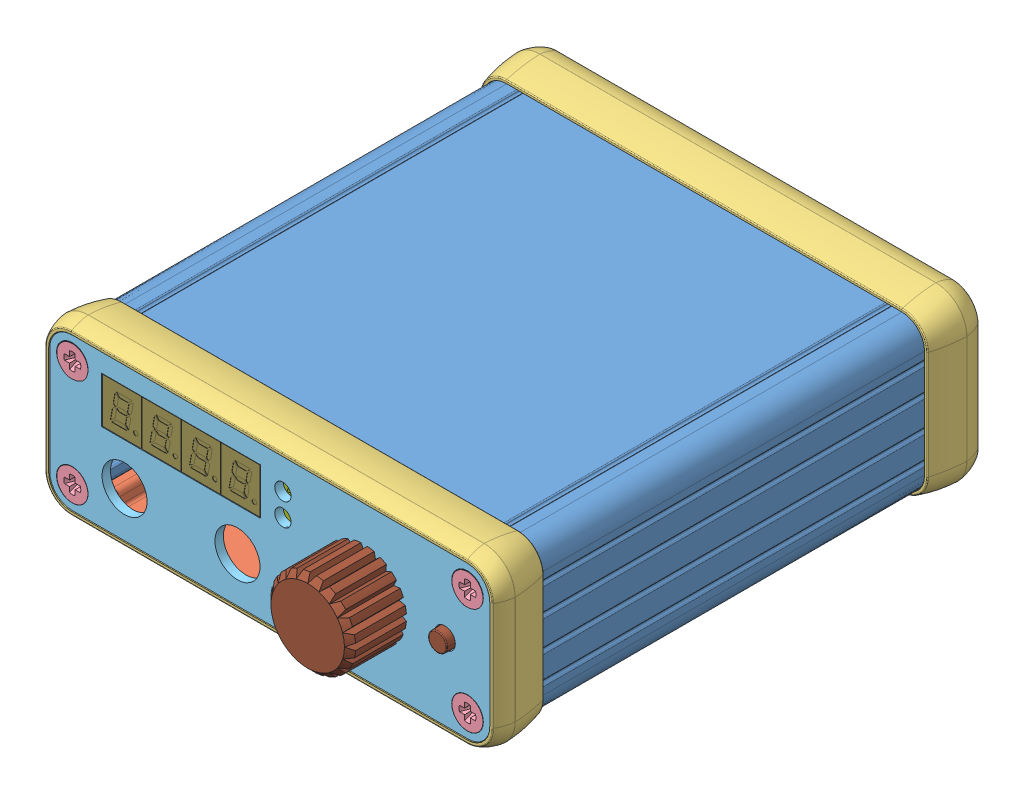
SolidWorks assembly Assembly_microbench_psu, configuration Standard. Lengths in mm.
Overall size (81.13 30.13 96.2).
1223 component instances, 156 part files, 17 mates.
Components (placement in the parent):
- 1455J801BK.step-1: 1455J801BK.step [Standard] at (-56.3915 -8.7776 0) size (81.13 30.13 86)
  - J Channel Extrusion 80mm.step-1: J Channel Extrusion 80mm.step [Standard] at origin size (78 27.01 80)
  - J Cap Extrusion 80mm.step-1: J Cap Extrusion 80mm.step [Standard] at (0 -27.01 0) size (66.9 4.29 80)
  - K Bezel.step-1: K Bezel.step [Standard] at (0 -13.4978 40) size (81.13 30.13 9)
  - K Bezel.step-2: K Bezel.step [Standard] at (0 -13.4978 -40) x (1 0 0) z (0 0 -1) size (81.13 30.13 9)
  - K1 End Panel.step-1: K1 End Panel.step [Standard] at (0.0215 -13.5485 41.4) size (77.98 26.92 1.5) (hidden)
  - K1 End Panel.step-2: K1 End Panel.step [Standard] at (-0.0215 -13.5485 -41.4) x (1 0 0) z (0 0 -1) size (77.98 26.92 1.5) (hidden)
  - 1455 screw.step-1: 1455 screw.step [Standard] at (-34.967 -4.087 42.9) x (1 0 0) z (0 0 -1) size (5.5 5.5 8)
  - 1455 screw.step-2: 1455 screw.step [Standard] at (-34.967 -23.01 42.9) x (1 0 0) z (0 0 -1) size (5.5 5.5 8)
  - 1455 screw.step-3: 1455 screw.step [Standard] at (35.01 -4.087 42.9) x (1 0 0) z (0 0 -1) size (5.5 5.5 8)
  - 1455 screw.step-4: 1455 screw.step [Standard] at (35.01 -23.01 42.9) x (1 0 0) z (0 0 -1) size (5.5 5.5 8)
  - 1455 screw.step-5: 1455 screw.step [Standard] at (34.967 -4.087 -42.9) size (5.5 5.5 8)
  - 1455 screw.step-6: 1455 screw.step [Standard] at (34.967 -23.01 -42.9) size (5.5 5.5 8)
  - 1455 screw.step-7: 1455 screw.step [Standard] at (-35.01 -4.087 -42.9) size (5.5 5.5 8)
  - 1455 screw.step-8: 1455 screw.step [Standard] at (-35.01 -23.01 -42.9) size (5.5 5.5 8)
- Front Cover-1: Front Cover [Standard] at (-95.3565 -35.7344 41.4) size (77.98 26.92 6.3)
- Back Cover-1: Back Cover [Standard] at (-95.3565 -35.7344 -42.9) size (77.98 26.92 1.5)
- display-board.step-1: display-board.step [Standard] at (-86.3675 -21.7604 39.8) size (43.75 11.2 5.28)
  - Board.step-1: Board.step [Standard] at origin size (43.75 11.2 1.42)
    - Open CASCADE STEP translator 7.5 4.1.1.step-1: Open CASCADE STEP translator 7.5 4.1.1.step [Standard] at (0 0 -1.4202) size (43.75 11.2 1.42)
  - D2.step-1: D2.step [Standard] at origin size (1.6 1.6 0.7)
    - 150066RG74000 (rev1)_RGB8421504.step-1: 150066RG74000 (rev1)_RGB8421504.step [Standard] at (32.25 3.6 0) x (0 1 0) z (0 0 1) size (1.6 1.6 0.7)
      - body.step-1: body.step [Standard] at origin size (1.6 1.6 0.3)
      - pole.step-1: pole.step [Standard] at origin size (1.31 1.26 0.3)
      - contact.step-1: contact.step [Standard] at origin size (1.6 1.6 0.53)
      - lense.step-1: lense.step [Standard] at (0 0.55 0.3) size (1.1 1.6 0.4)
  - DS4.step-1: DS4.step [Standard] at origin size (6.9 10 3.05)
    - ACSX02-41_RGB8421504.step-1: ACSX02-41_RGB8421504.step [Standard] at (24.75 5.6 3.0627) x (1 0 0) z (0 -1 0) size (6.9 3.05 10)
  - DS3.step-1: DS3.step [Standard] at origin size (6.9 10 3.05)
    - ACSX02-41_RGB8421504.step-1: ACSX02-41_RGB8421504.step [Standard] at (17.75 5.6 3.0627) x (1 0 0) z (0 -1 0) size (6.9 3.05 10)
  - DS2.step-1: DS2.step [Standard] at origin size (6.9 10 3.05)
    - ACSX02-41_RGB8421504.step-1: ACSX02-41_RGB8421504.step [Standard] at (10.75 5.6 3.0627) x (1 0 0) z (0 -1 0) size (6.9 3.05 10)
  - DS1.step-1: DS1.step [Standard] at origin size (6.9 10 3.05)
    - ACSX02-41_RGB8421504.step-1: ACSX02-41_RGB8421504.step [Standard] at (3.75 5.6 3.0627) x (1 0 0) z (0 -1 0) size (6.9 3.05 10)
  - D1.step-1: D1.step [Standard] at origin size (1.6 1.6 0.7)
    - 150066RG74000 (rev1)_RGB8421504.step-1: 150066RG74000 (rev1)_RGB8421504.step [Standard] at (32.25 7.6 0) x (0 -1 0) z (0 0 1) size (1.6 1.6 0.7)
      - body.step-1: body.step [Standard] at origin size (1.6 1.6 0.3)
      - pole.step-1: pole.step [Standard] at origin size (1.31 1.26 0.3)
      - contact.step-1: contact.step [Standard] at origin size (1.6 1.6 0.53)
      - lense.step-1: lense.step [Standard] at (0 0.55 0.3) size (1.1 1.6 0.4)
  - C4.step-1: C4.step [Standard] at origin size (1.27 1.27 0.65)
    - 5696318048.step-1: 5696318048.step [Standard] at (10.25 7.35 -1.4202) x (-0.707107 -0.707107 0) z (0 0 -1) size (1.15 0.65 0.65)
      - Terminal.step-1: Terminal.step [Standard] at (-0.575 -0.325 0) size (1.15 0.65 0.65)
        - Open CASCADE STEP translator 6.8 5.1.1.step-1: Open CASCADE STEP translator 6.8 5.1.1.step [Standard] at origin size (0.15 0.65 0.65)
        - Open CASCADE STEP translator 6.8 5.1.2.step-1: Open CASCADE STEP translator 6.8 5.1.2.step [Standard] at origin size (0.15 0.65 0.65)
      - Mid_Body.step-1: Mid_Body.step [Standard] at (-0.575 -0.325 0) size (0.85 0.65 0.65)
        - Open CASCADE STEP translator 6.8 5.2.1.step-1: Open CASCADE STEP translator 6.8 5.2.1.step [Standard] at origin size (0.85 0.65 0.65)
  - C3.step-1: C3.step [Standard] at origin size (0.65 1.15 0.65)
    - 7876647632.step-1: 7876647632.step [Standard] at (19.25 5.85 -1.4202) x (0 1 0) z (0 0 -1) size (1.15 0.65 0.65)
      - Terminal-1.step-1: Terminal-1.step [Standard] at (-0.575 -0.325 0) size (1.15 0.65 0.65)
        - Open CASCADE STEP translator 6.8 5.1.1-0.step-1: Open CASCADE STEP translator 6.8 5.1.1-0.step [Standard] at origin size (0.15 0.65 0.65)
        - Open CASCADE STEP translator 6.8 5.1.2-1.step-1: Open CASCADE STEP translator 6.8 5.1.2-1.step [Standard] at origin size (0.15 0.65 0.65)
      - Mid_Body-1.step-1: Mid_Body-1.step [Standard] at (-0.575 -0.325 0) size (0.85 0.65 0.65)
        - Open CASCADE STEP translator 6.8 5.2.1-2.step-1: Open CASCADE STEP translator 6.8 5.2.1-2.step [Standard] at origin size (0.85 0.65 0.65)
  - C2.step-1: C2.step [Standard] at origin size (0.9 1.7 0.55)
    - 7556045440.step-1: 7556045440.step [Standard] at (20.5 5.85 -1.4202) x (0 1 0) z (0 0 -1) size (1.7 0.9 0.55)
      - Terminal-2.step-1: Terminal-2.step [Standard] at (-0.85 -0.45 0) size (0.1 0.9 0.55)
        - Open CASCADE STEP translator 7.5 6.2.1.step-1: Open CASCADE STEP translator 7.5 6.2.1.step [Standard] at origin size (0.1 0.9 0.55)
      - Terminal-2.step-2: Terminal-2.step [Standard] at (0.85 0.45 0) x (-1 0 0) z (0 0 1) size (0.1 0.9 0.55)
        - Open CASCADE STEP translator 7.5 6.2.1.step-1: Open CASCADE STEP translator 7.5 6.2.1.step [Standard] at origin size (0.1 0.9 0.55)
      - Mid Body.step-1: Mid Body.step [Standard] at (-0.85 -0.45 0) size (1.59 0.9 0.44)
      - Mark.step-1: Mark.step [Standard] at (-0.75 -0.45 0.495) size (1.5 0.9 0.06)
  - IC1.step-1: IC1.step [Standard] at origin size (5.8 5.8 0.8)
    - 5696319008.step-1: 5696319008.step [Standard] at (14.25 5.6 -1.4202) x (0.707107 -0.707107 0) z (0 0 -1) size (4.1 4.1 0.8)
      - Body.step-1: Body.step [Standard] at (-2.05 -2.05 0) size (4.1 4.1 0.8)
        - Open CASCADE STEP translator 7.5 1.2.1.step-1: Open CASCADE STEP translator 7.5 1.2.1.step [Standard] at origin size (4.1 4.1 0.8)
      - Pin Shape.step-1: Pin Shape.step [Standard] at (-2.05 -1.37 0) size (0.4 0.24 0.2)
        - Open CASCADE STEP translator 7.5 1.4.1.step-1: Open CASCADE STEP translator 7.5 1.4.1.step [Standard] at origin size (0.4 0.24 0.2)
      - Pin Shape.step-2: Pin Shape.step [Standard] at (2.05 1.37 0) x (-1 0 0) z (0 0 1) size (0.4 0.24 0.2)
        - Open CASCADE STEP translator 7.5 1.4.1.step-1: Open CASCADE STEP translator 7.5 1.4.1.step [Standard] at origin size (0.4 0.24 0.2)
      - Pin Shape.step-3: Pin Shape.step [Standard] at (-2.05 -0.87 0) size (0.4 0.24 0.2)
        - Open CASCADE STEP translator 7.5 1.4.1.step-1: Open CASCADE STEP translator 7.5 1.4.1.step [Standard] at origin size (0.4 0.24 0.2)
      - Pin Shape.step-4: Pin Shape.step [Standard] at (2.05 0.87 0) x (-1 0 0) z (0 0 1) size (0.4 0.24 0.2)
        - Open CASCADE STEP translator 7.5 1.4.1.step-1: Open CASCADE STEP translator 7.5 1.4.1.step [Standard] at origin size (0.4 0.24 0.2)
      - Pin Shape.step-5: Pin Shape.step [Standard] at (-2.05 -0.37 0) size (0.4 0.24 0.2)
        - Open CASCADE STEP translator 7.5 1.4.1.step-1: Open CASCADE STEP translator 7.5 1.4.1.step [Standard] at origin size (0.4 0.24 0.2)
      - Pin Shape.step-6: Pin Shape.step [Standard] at (2.05 0.37 0) x (-1 0 0) z (0 0 1) size (0.4 0.24 0.2)
        - Open CASCADE STEP translator 7.5 1.4.1.step-1: Open CASCADE STEP translator 7.5 1.4.1.step [Standard] at origin size (0.4 0.24 0.2)
      - Pin Shape.step-7: Pin Shape.step [Standard] at (-2.05 0.13 0) size (0.4 0.24 0.2)
        - Open CASCADE STEP translator 7.5 1.4.1.step-1: Open CASCADE STEP translator 7.5 1.4.1.step [Standard] at origin size (0.4 0.24 0.2)
      - Pin Shape.step-8: Pin Shape.step [Standard] at (2.05 -0.13 0) x (-1 0 0) z (0 0 1) size (0.4 0.24 0.2)
        - Open CASCADE STEP translator 7.5 1.4.1.step-1: Open CASCADE STEP translator 7.5 1.4.1.step [Standard] at origin size (0.4 0.24 0.2)
      - Pin Shape.step-9: Pin Shape.step [Standard] at (-2.05 0.63 0) size (0.4 0.24 0.2)
        - Open CASCADE STEP translator 7.5 1.4.1.step-1: Open CASCADE STEP translator 7.5 1.4.1.step [Standard] at origin size (0.4 0.24 0.2)
      - Pin Shape.step-10: Pin Shape.step [Standard] at (2.05 -0.63 0) x (-1 0 0) z (0 0 1) size (0.4 0.24 0.2)
        - Open CASCADE STEP translator 7.5 1.4.1.step-1: Open CASCADE STEP translator 7.5 1.4.1.step [Standard] at origin size (0.4 0.24 0.2)
      - Pin Shape.step-11: Pin Shape.step [Standard] at (-2.05 1.13 0) size (0.4 0.24 0.2)
        - Open CASCADE STEP translator 7.5 1.4.1.step-1: Open CASCADE STEP translator 7.5 1.4.1.step [Standard] at origin size (0.4 0.24 0.2)
      - Pin Shape.step-12: Pin Shape.step [Standard] at (2.05 -1.13 0) x (-1 0 0) z (0 0 1) size (0.4 0.24 0.2)
        - Open CASCADE STEP translator 7.5 1.4.1.step-1: Open CASCADE STEP translator 7.5 1.4.1.step [Standard] at origin size (0.4 0.24 0.2)
      - Pin Shape.step-13: Pin Shape.step [Standard] at (-1.13 -2.05 0) x (0 1 0) z (0 0 1) size (0.4 0.24 0.2)
        - Open CASCADE STEP translator 7.5 1.4.1.step-1: Open CASCADE STEP translator 7.5 1.4.1.step [Standard] at origin size (0.4 0.24 0.2)
      - Pin Shape.step-14: Pin Shape.step [Standard] at (1.13 2.05 0) x (0 -1 0) z (0 0 1) size (0.4 0.24 0.2)
        - Open CASCADE STEP translator 7.5 1.4.1.step-1: Open CASCADE STEP translator 7.5 1.4.1.step [Standard] at origin size (0.4 0.24 0.2)
      - Pin Shape.step-15: Pin Shape.step [Standard] at (-0.63 -2.05 0) x (0 1 0) z (0 0 1) size (0.4 0.24 0.2)
        - Open CASCADE STEP translator 7.5 1.4.1.step-1: Open CASCADE STEP translator 7.5 1.4.1.step [Standard] at origin size (0.4 0.24 0.2)
      - Pin Shape.step-16: Pin Shape.step [Standard] at (0.63 2.05 0) x (0 -1 0) z (0 0 1) size (0.4 0.24 0.2)
        - Open CASCADE STEP translator 7.5 1.4.1.step-1: Open CASCADE STEP translator 7.5 1.4.1.step [Standard] at origin size (0.4 0.24 0.2)
      - Pin Shape.step-17: Pin Shape.step [Standard] at (-0.13 -2.05 0) x (0 1 0) z (0 0 1) size (0.4 0.24 0.2)
        - Open CASCADE STEP translator 7.5 1.4.1.step-1: Open CASCADE STEP translator 7.5 1.4.1.step [Standard] at origin size (0.4 0.24 0.2)
      - Pin Shape.step-18: Pin Shape.step [Standard] at (0.13 2.05 0) x (0 -1 0) z (0 0 1) size (0.4 0.24 0.2)
        - Open CASCADE STEP translator 7.5 1.4.1.step-1: Open CASCADE STEP translator 7.5 1.4.1.step [Standard] at origin size (0.4 0.24 0.2)
      - Pin Shape.step-19: Pin Shape.step [Standard] at (0.37 -2.05 0) x (0 1 0) z (0 0 1) size (0.4 0.24 0.2)
        - Open CASCADE STEP translator 7.5 1.4.1.step-1: Open CASCADE STEP translator 7.5 1.4.1.step [Standard] at origin size (0.4 0.24 0.2)
      - Pin Shape.step-20: Pin Shape.step [Standard] at (-0.37 2.05 0) x (0 -1 0) z (0 0 1) size (0.4 0.24 0.2)
        - Open CASCADE STEP translator 7.5 1.4.1.step-1: Open CASCADE STEP translator 7.5 1.4.1.step [Standard] at origin size (0.4 0.24 0.2)
      - Pin Shape.step-21: Pin Shape.step [Standard] at (0.87 -2.05 0) x (0 1 0) z (0 0 1) size (0.4 0.24 0.2)
        - Open CASCADE STEP translator 7.5 1.4.1.step-1: Open CASCADE STEP translator 7.5 1.4.1.step [Standard] at origin size (0.4 0.24 0.2)
      - Pin Shape.step-22: Pin Shape.step [Standard] at (-0.87 2.05 0) x (0 -1 0) z (0 0 1) size (0.4 0.24 0.2)
        - Open CASCADE STEP translator 7.5 1.4.1.step-1: Open CASCADE STEP translator 7.5 1.4.1.step [Standard] at origin size (0.4 0.24 0.2)
      - Pin Shape.step-23: Pin Shape.step [Standard] at (1.37 -2.05 0) x (0 1 0) z (0 0 1) size (0.4 0.24 0.2)
        - Open CASCADE STEP translator 7.5 1.4.1.step-1: Open CASCADE STEP translator 7.5 1.4.1.step [Standard] at origin size (0.4 0.24 0.2)
      - Pin Shape.step-24: Pin Shape.step [Standard] at (-1.37 2.05 0) x (0 -1 0) z (0 0 1) size (0.4 0.24 0.2)
        - Open CASCADE STEP translator 7.5 1.4.1.step-1: Open CASCADE STEP translator 7.5 1.4.1.step [Standard] at origin size (0.4 0.24 0.2)
      - Open CASCADE STEP translator 7.5 1.1.step-1: Open CASCADE STEP translator 7.5 1.1.step [Standard] at (-2.05 -2.05 0) size (0.52 0.52 0.01)
      - Thermal Shape.step-1: Thermal Shape.step [Standard] at (-1.275 -1.275 -0.001) size (2.55 2.55 0)
  - C1.step-1: C1.step [Standard] at origin size (1.21 2.01 0.72)
    - RC0805N.step-1: RC0805N.step [Standard] at (22.2501 5.8501 -1.4082) x (0 1 0) z (0 0 -1) size (2.01 1.21 0.72)
- ui-board.step-1: ui-board.step [Standard] at (-48.1285 -32.2724 36.6) size (30.5 20 16.19)
  - Board.step-1: Board.step [Standard] at origin size (30.5 20 1.42)
    - Open CASCADE STEP translator 7.5 2.1.1.step-1: Open CASCADE STEP translator 7.5 2.1.1.step [Standard] at (0 0 -1.4202) size (30.5 20 1.42)
  - SW1.step-1: SW1.step [Standard] at origin size (15.01 18.01 15.31)
    - PEC11S-929K-S0015_RGB8421504.step-1: PEC11S-929K-S0015_RGB8421504.step [Standard] at (6.9669 13.8225 -0.2873) size (15.01 18.01 15.31)
  - SW.step-1: SW.step [Standard] at origin size (6 10 7.6)
    - Same_Sky_TS04-66-75-BK-160-SMT_RGB8421504.step-1: Same_Sky_TS04-66-75-BK-160-SMT_RGB8421504.step [Standard] at (22.75 10 0.1127) x (0 1 0) z (1 0 0) size (10 7.6 6)
  - R6.step-1: R6.step [Standard] at origin size (0.55 1.1 0.4)
    - 7876642432.step-1: 7876642432.step [Standard] at (24.25 9.5 -1.4202) x (0 -1 0) z (0 0 -1) size (1.1 0.55 0.4)
      - Terminal.step-1: Terminal.step [Standard] at (-0.55 -0.275 0) size (0.15 0.55 0.4)
        - Open CASCADE STEP translator 6.8 6.2.1.step-1: Open CASCADE STEP translator 6.8 6.2.1.step [Standard] at origin size (0.15 0.55 0.4)
      - Terminal.step-2: Terminal.step [Standard] at (0.55 0.275 0) x (-1 0 0) z (0 0 1) size (0.15 0.55 0.4)
        - Open CASCADE STEP translator 6.8 6.2.1.step-1: Open CASCADE STEP translator 6.8 6.2.1.step [Standard] at origin size (0.15 0.55 0.4)
      - Mid_Body.step-1: Mid_Body.step [Standard] at (-0.55 -0.275 0) size (1.02 0.55 0.32)
      - Mark.step-1: Mark.step [Standard] at (-0.4 -0.275 0.36) size (0.8 0.55 0.04)
  - R5.step-1: R5.step [Standard] at origin size (1.1 0.55 0.4)
    - 7876648592.step-1: 7876648592.step [Standard] at (14.5 9 -1.4202) x (-1 0 0) z (0 0 -1) size (1.1 0.55 0.4)
      - Terminal-1.step-1: Terminal-1.step [Standard] at (-0.55 -0.275 0) size (0.15 0.55 0.4)
        - Open CASCADE STEP translator 6.8 6.2.1-0.step-1: Open CASCADE STEP translator 6.8 6.2.1-0.step [Standard] at origin size (0.15 0.55 0.4)
      - Terminal-1.step-2: Terminal-1.step [Standard] at (0.55 0.275 0) x (-1 0 0) z (0 0 1) size (0.15 0.55 0.4)
        - Open CASCADE STEP translator 6.8 6.2.1-0.step-1: Open CASCADE STEP translator 6.8 6.2.1-0.step [Standard] at origin size (0.15 0.55 0.4)
      - Mid_Body-1.step-1: Mid_Body-1.step [Standard] at (-0.55 -0.275 0) size (1.02 0.55 0.32)
      - Mark-2.step-1: Mark-2.step [Standard] at (-0.4 -0.275 0.36) size (0.8 0.55 0.04)
  - R4.step-1: R4.step [Standard] at origin size (1.1 0.55 0.4)
    - 7876648592.step-1: 7876648592.step [Standard] at (14.5 8 -1.4202) x (-1 0 0) z (0 0 -1) size (1.1 0.55 0.4)
      - Terminal-1.step-1: Terminal-1.step [Standard] at (-0.55 -0.275 0) size (0.15 0.55 0.4)
        - Open CASCADE STEP translator 6.8 6.2.1-0.step-1: Open CASCADE STEP translator 6.8 6.2.1-0.step [Standard] at origin size (0.15 0.55 0.4)
      - Terminal-1.step-2: Terminal-1.step [Standard] at (0.55 0.275 0) x (-1 0 0) z (0 0 1) size (0.15 0.55 0.4)
        - Open CASCADE STEP translator 6.8 6.2.1-0.step-1: Open CASCADE STEP translator 6.8 6.2.1-0.step [Standard] at origin size (0.15 0.55 0.4)
      - Mid_Body-1.step-1: Mid_Body-1.step [Standard] at (-0.55 -0.275 0) size (1.02 0.55 0.32)
      - Mark-2.step-1: Mark-2.step [Standard] at (-0.4 -0.275 0.36) size (0.8 0.55 0.04)
  - R3.step-1: R3.step [Standard] at origin size (0.55 1.1 0.4)
    - 7876642432.step-1: 7876642432.step [Standard] at (16 13 -1.4202) x (0 -1 0) z (0 0 -1) size (1.1 0.55 0.4)
      - Terminal.step-1: Terminal.step [Standard] at (-0.55 -0.275 0) size (0.15 0.55 0.4)
        - Open CASCADE STEP translator 6.8 6.2.1.step-1: Open CASCADE STEP translator 6.8 6.2.1.step [Standard] at origin size (0.15 0.55 0.4)
      - Terminal.step-2: Terminal.step [Standard] at (0.55 0.275 0) x (-1 0 0) z (0 0 1) size (0.15 0.55 0.4)
        - Open CASCADE STEP translator 6.8 6.2.1.step-1: Open CASCADE STEP translator 6.8 6.2.1.step [Standard] at origin size (0.15 0.55 0.4)
      - Mid_Body.step-1: Mid_Body.step [Standard] at (-0.55 -0.275 0) size (1.02 0.55 0.32)
      - Mark.step-1: Mark.step [Standard] at (-0.4 -0.275 0.36) size (0.8 0.55 0.04)
  - R2.step-1: R2.step [Standard] at origin size (0.55 1.1 0.4)
    - 7876642992.step-1: 7876642992.step [Standard] at (13 10.25 -1.4202) x (0 1 0) z (0 0 -1) size (1.1 0.55 0.4)
      - Terminal-2.step-1: Terminal-2.step [Standard] at (-0.55 -0.275 0) size (0.15 0.55 0.4)
        - Open CASCADE STEP translator 6.8 6.2.1-3.step-1: Open CASCADE STEP translator 6.8 6.2.1-3.step [Standard] at origin size (0.15 0.55 0.4)
      - Terminal-2.step-2: Terminal-2.step [Standard] at (0.55 0.275 0) x (-1 0 0) z (0 0 1) size (0.15 0.55 0.4)
        - Open CASCADE STEP translator 6.8 6.2.1-3.step-1: Open CASCADE STEP translator 6.8 6.2.1-3.step [Standard] at origin size (0.15 0.55 0.4)
      - Mid_Body-4.step-1: Mid_Body-4.step [Standard] at (-0.55 -0.275 0) size (1.02 0.55 0.32)
      - Mark-5.step-1: Mark-5.step [Standard] at (-0.4 -0.275 0.36) size (0.8 0.55 0.04)
  - R1.step-1: R1.step [Standard] at origin size (0.55 1.1 0.4)
    - 7876642432.step-1: 7876642432.step [Standard] at (13 6.5 -1.4202) x (0 -1 0) z (0 0 -1) size (1.1 0.55 0.4)
      - Terminal.step-1: Terminal.step [Standard] at (-0.55 -0.275 0) size (0.15 0.55 0.4)
        - Open CASCADE STEP translator 6.8 6.2.1.step-1: Open CASCADE STEP translator 6.8 6.2.1.step [Standard] at origin size (0.15 0.55 0.4)
      - Terminal.step-2: Terminal.step [Standard] at (0.55 0.275 0) x (-1 0 0) z (0 0 1) size (0.15 0.55 0.4)
        - Open CASCADE STEP translator 6.8 6.2.1.step-1: Open CASCADE STEP translator 6.8 6.2.1.step [Standard] at origin size (0.15 0.55 0.4)
      - Mid_Body.step-1: Mid_Body.step [Standard] at (-0.55 -0.275 0) size (1.02 0.55 0.32)
      - Mark.step-1: Mark.step [Standard] at (-0.4 -0.275 0.36) size (0.8 0.55 0.04)
  - C4.step-1: C4.step [Standard] at origin size (0.65 1.15 0.65)
    - 7876639952.step-1: 7876639952.step [Standard] at (24.25 11.5 -1.4202) x (0 -1 0) z (0 0 -1) size (1.15 0.65 0.65)
      - Terminal-3.step-1: Terminal-3.step [Standard] at (-0.575 -0.325 0) size (1.15 0.65 0.65)
        - Open CASCADE STEP translator 6.8 5.1.1.step-1: Open CASCADE STEP translator 6.8 5.1.1.step [Standard] at origin size (0.15 0.65 0.65)
        - Open CASCADE STEP translator 6.8 5.1.2.step-1: Open CASCADE STEP translator 6.8 5.1.2.step [Standard] at origin size (0.15 0.65 0.65)
      - Mid_Body-6.step-1: Mid_Body-6.step [Standard] at (-0.575 -0.325 0) size (0.85 0.65 0.65)
        - Open CASCADE STEP translator 6.8 5.2.1.step-1: Open CASCADE STEP translator 6.8 5.2.1.step [Standard] at origin size (0.85 0.65 0.65)
  - C3.step-1: C3.step [Standard] at origin size (0.65 1.15 0.65)
    - 7876647632.step-1: 7876647632.step [Standard] at (16 6.5 -1.4202) x (0 1 0) z (0 0 -1) size (1.15 0.65 0.65)
      - Terminal-4.step-1: Terminal-4.step [Standard] at (-0.575 -0.325 0) size (1.15 0.65 0.65)
        - Open CASCADE STEP translator 6.8 5.1.1-7.step-1: Open CASCADE STEP translator 6.8 5.1.1-7.step [Standard] at origin size (0.15 0.65 0.65)
        - Open CASCADE STEP translator 6.8 5.1.2-8.step-1: Open CASCADE STEP translator 6.8 5.1.2-8.step [Standard] at origin size (0.15 0.65 0.65)
      - Mid_Body-1-9.step-1: Mid_Body-1-9.step [Standard] at (-0.575 -0.325 0) size (0.85 0.65 0.65)
        - Open CASCADE STEP translator 6.8 5.2.1-10.step-1: Open CASCADE STEP translator 6.8 5.2.1-10.step [Standard] at origin size (0.85 0.65 0.65)
  - C2.step-1: C2.step [Standard] at origin size (0.65 1.15 0.65)
    - 7876639952.step-1: 7876639952.step [Standard] at (16 10.25 -1.4202) x (0 -1 0) z (0 0 -1) size (1.15 0.65 0.65)
      - Terminal-3.step-1: Terminal-3.step [Standard] at (-0.575 -0.325 0) size (1.15 0.65 0.65)
        - Open CASCADE STEP translator 6.8 5.1.1.step-1: Open CASCADE STEP translator 6.8 5.1.1.step [Standard] at origin size (0.15 0.65 0.65)
        - Open CASCADE STEP translator 6.8 5.1.2.step-1: Open CASCADE STEP translator 6.8 5.1.2.step [Standard] at origin size (0.15 0.65 0.65)
      - Mid_Body-6.step-1: Mid_Body-6.step [Standard] at (-0.575 -0.325 0) size (0.85 0.65 0.65)
        - Open CASCADE STEP translator 6.8 5.2.1.step-1: Open CASCADE STEP translator 6.8 5.2.1.step [Standard] at origin size (0.85 0.65 0.65)
  - C1.step-1: C1.step [Standard] at origin size (0.65 1.15 0.65)
    - 7876639952.step-1: 7876639952.step [Standard] at (16 15 -1.4202) x (0 -1 0) z (0 0 -1) size (1.15 0.65 0.65)
      - Terminal-3.step-1: Terminal-3.step [Standard] at (-0.575 -0.325 0) size (1.15 0.65 0.65)
        - Open CASCADE STEP translator 6.8 5.1.1.step-1: Open CASCADE STEP translator 6.8 5.1.1.step [Standard] at origin size (0.15 0.65 0.65)
        - Open CASCADE STEP translator 6.8 5.1.2.step-1: Open CASCADE STEP translator 6.8 5.1.2.step [Standard] at origin size (0.15 0.65 0.65)
      - Mid_Body-6.step-1: Mid_Body-6.step [Standard] at (-0.575 -0.325 0) size (0.85 0.65 0.65)
        - Open CASCADE STEP translator 6.8 5.2.1.step-1: Open CASCADE STEP translator 6.8 5.2.1.step [Standard] at origin size (0.85 0.65 0.65)
- main-board.step-1: main-board.step [Standard] at (-93.8915 -23.4474 -41.4) x (0 0 1) z (0 1 0) size (82.8 75 12.43)
  - Board.step-1: Board.step [Standard] at origin size (82.8 75 1.42)
    - Open CASCADE STEP translator 7.5 3.1.1.step-1: Open CASCADE STEP translator 7.5 3.1.1.step [Standard] at (0 0 -1.4202) size (82.8 75 1.42)
  - R100.step-1: R100.step [Standard] at origin size (1.1 0.55 0.4)
    - 7876648592.step-1: 7876648592.step [Standard] at (57.3 61.6 0) x (-1 0 0) z (0 0 1) size (1.1 0.55 0.4)
      - Terminal.step-1: Terminal.step [Standard] at (-0.55 -0.275 0) size (0.15 0.55 0.4)
        - Open CASCADE STEP translator 6.8 6.2.1.step-1: Open CASCADE STEP translator 6.8 6.2.1.step [Standard] at origin size (0.15 0.55 0.4)
      - Terminal.step-2: Terminal.step [Standard] at (0.55 0.275 0) x (-1 0 0) z (0 0 1) size (0.15 0.55 0.4)
        - Open CASCADE STEP translator 6.8 6.2.1.step-1: Open CASCADE STEP translator 6.8 6.2.1.step [Standard] at origin size (0.15 0.55 0.4)
      - Mid_Body.step-1: Mid_Body.step [Standard] at (-0.55 -0.275 0) size (1.02 0.55 0.32)
      - Mark.step-1: Mark.step [Standard] at (-0.4 -0.275 0.36) size (0.8 0.55 0.04)
  - C516.step-1: C516.step [Standard] at origin size (1.15 0.65 0.65)
    - 7556052240.step-1: 7556052240.step [Standard] at (31.95 17.45 0) x (-1 0 0) z (0 0 1) size (1.15 0.65 0.65)
      - Terminal-1.step-1: Terminal-1.step [Standard] at (-0.575 -0.325 0) size (1.15 0.65 0.65)
        - Open CASCADE STEP translator 6.8 5.1.1.step-1: Open CASCADE STEP translator 6.8 5.1.1.step [Standard] at origin size (0.15 0.65 0.65)
        - Open CASCADE STEP translator 6.8 5.1.2.step-1: Open CASCADE STEP translator 6.8 5.1.2.step [Standard] at origin size (0.15 0.65 0.65)
      - Mid_Body-0.step-1: Mid_Body-0.step [Standard] at (-0.575 -0.325 0) size (0.85 0.65 0.65)
        - Open CASCADE STEP translator 6.8 5.2.1.step-1: Open CASCADE STEP translator 6.8 5.2.1.step [Standard] at origin size (0.85 0.65 0.65)
  - C515.step-1: C515.step [Standard] at origin size (1.15 0.65 0.65)
    - 7556052240.step-1: 7556052240.step [Standard] at (31.95 18.75 0) x (-1 0 0) z (0 0 1) size (1.15 0.65 0.65)
      - Terminal-1.step-1: Terminal-1.step [Standard] at (-0.575 -0.325 0) size (1.15 0.65 0.65)
        - Open CASCADE STEP translator 6.8 5.1.1.step-1: Open CASCADE STEP translator 6.8 5.1.1.step [Standard] at origin size (0.15 0.65 0.65)
        - Open CASCADE STEP translator 6.8 5.1.2.step-1: Open CASCADE STEP translator 6.8 5.1.2.step [Standard] at origin size (0.15 0.65 0.65)
      - Mid_Body-0.step-1: Mid_Body-0.step [Standard] at (-0.575 -0.325 0) size (0.85 0.65 0.65)
        - Open CASCADE STEP translator 6.8 5.2.1.step-1: Open CASCADE STEP translator 6.8 5.2.1.step [Standard] at origin size (0.85 0.65 0.65)
  - C504.step-1: C504.step [Standard] at origin size (10.3 11 10)
    - ChemiCon_JA0_RGB8421504.step-1: ChemiCon_JA0_RGB8421504.step [Standard] at (5.6 39.5 0) x (0 1 0) z (0 0 1) size (11 10.3 10)
      - E-CHIP_D10_L10_ELEMENT.step-1: E-CHIP_D10_L10_ELEMENT.step [Standard] at origin size (10 10 9.35)
      - E-CHIP_D10_LEAD-.step-1: E-CHIP_D10_LEAD-.step [Standard] at origin size (3.26 0.91 2)
      - E-CHIP_D10_LEAD+.step-1: E-CHIP_D10_LEAD+.step [Standard] at origin size (3.26 0.91 2)
      - E-CHIP_D10_TABLE.step-1: E-CHIP_D10_TABLE.step [Standard] at origin size (10.3 10.3 2.31)
  - C500.step-1: C500.step [Standard] at origin size (1.15 0.65 0.65)
    - 7556050560.step-1: 7556050560.step [Standard] at (23.6 35.2 0) x (1 0 0) z (0 0 1) size (1.15 0.65 0.65)
      - Terminal-2.step-1: Terminal-2.step [Standard] at (-0.575 -0.325 0) size (1.15 0.65 0.65)
        - Open CASCADE STEP translator 6.8 5.1.1-1.step-1: Open CASCADE STEP translator 6.8 5.1.1-1.step [Standard] at origin size (0.15 0.65 0.65)
        - Open CASCADE STEP translator 6.8 5.1.2-2.step-1: Open CASCADE STEP translator 6.8 5.1.2-2.step [Standard] at origin size (0.15 0.65 0.65)
      - Mid_Body-1.step-1: Mid_Body-1.step [Standard] at (-0.575 -0.325 0) size (0.85 0.65 0.65)
        - Open CASCADE STEP translator 6.8 5.2.1-3.step-1: Open CASCADE STEP translator 6.8 5.2.1-3.step [Standard] at origin size (0.85 0.65 0.65)
  - C501.step-1: C501.step [Standard] at origin size (0.65 1.15 0.65)
    - 7876639952.step-1: 7876639952.step [Standard] at (16 43 0) x (0 1 0) z (0 0 1) size (1.15 0.65 0.65)
      - Terminal-3.step-1: Terminal-3.step [Standard] at (-0.575 -0.325 0) size (1.15 0.65 0.65)
        - Open CASCADE STEP translator 6.8 5.1.1-4.step-1: Open CASCADE STEP translator 6.8 5.1.1-4.step [Standard] at origin size (0.15 0.65 0.65)
        - Open CASCADE STEP translator 6.8 5.1.2-5.step-1: Open CASCADE STEP translator 6.8 5.1.2-5.step [Standard] at origin size (0.15 0.65 0.65)
      - Mid_Body-2.step-1: Mid_Body-2.step [Standard] at (-0.575 -0.325 0) size (0.85 0.65 0.65)
        - Open CASCADE STEP translator 6.8 5.2.1-6.step-1: Open CASCADE STEP translator 6.8 5.2.1-6.step [Standard] at origin size (0.85 0.65 0.65)
  - C502.step-1: C502.step [Standard] at origin size (1.15 0.65 0.65)
    - 7556050560.step-1: 7556050560.step [Standard] at (20 35.2 0) x (1 0 0) z (0 0 1) size (1.15 0.65 0.65)
      - Terminal-2.step-1: Terminal-2.step [Standard] at (-0.575 -0.325 0) size (1.15 0.65 0.65)
        - Open CASCADE STEP translator 6.8 5.1.1-1.step-1: Open CASCADE STEP translator 6.8 5.1.1-1.step [Standard] at origin size (0.15 0.65 0.65)
        - Open CASCADE STEP translator 6.8 5.1.2-2.step-1: Open CASCADE STEP translator 6.8 5.1.2-2.step [Standard] at origin size (0.15 0.65 0.65)
      - Mid_Body-1.step-1: Mid_Body-1.step [Standard] at (-0.575 -0.325 0) size (0.85 0.65 0.65)
        - Open CASCADE STEP translator 6.8 5.2.1-3.step-1: Open CASCADE STEP translator 6.8 5.2.1-3.step [Standard] at origin size (0.85 0.65 0.65)
  - C505.step-1: C505.step [Standard] at origin size (1.45 2.2 1.45)
    - 7556051680.step-1: 7556051680.step [Standard] at (12.1 43.2 0) x (0 -1 0) z (0 0 1) size (2.2 1.45 1.45)
      - Terminal-4.step-1: Terminal-4.step [Standard] at (-1.1 -0.725 0) size (2.2 1.45 1.45)
        - Open CASCADE STEP translator 7.5 2.1.1.step-1: Open CASCADE STEP translator 7.5 2.1.1.step [Standard] at origin size (0.2 1.45 1.45)
        - Open CASCADE STEP translator 7.5 2.1.2.step-1: Open CASCADE STEP translator 7.5 2.1.2.step [Standard] at origin size (0.2 1.45 1.45)
      - Mid Body.step-1: Mid Body.step [Standard] at (-1.1 -0.725 0) size (1.8 1.45 1.45)
        - Open CASCADE STEP translator 7.5 2.2.1.step-1: Open CASCADE STEP translator 7.5 2.2.1.step [Standard] at origin size (1.8 1.45 1.45)
  - C511.step-1: C511.step [Standard] at origin size (0.9 1.7 0.55)
    - 7556045440.step-1: 7556045440.step [Standard] at (20.4 42.8 0) x (0 -1 0) z (0 0 1) size (1.7 0.9 0.55)
      - Terminal-5.step-1: Terminal-5.step [Standard] at (-0.85 -0.45 0) size (0.1 0.9 0.55)
        - Open CASCADE STEP translator 7.5 6.2.1.step-1: Open CASCADE STEP translator 7.5 6.2.1.step [Standard] at origin size (0.1 0.9 0.55)
      - Terminal-5.step-2: Terminal-5.step [Standard] at (0.85 0.45 0) x (-1 0 0) z (0 0 1) size (0.1 0.9 0.55)
        - Open CASCADE STEP translator 7.5 6.2.1.step-1: Open CASCADE STEP translator 7.5 6.2.1.step [Standard] at origin size (0.1 0.9 0.55)
      - Mid Body-7.step-1: Mid Body-7.step [Standard] at (-0.85 -0.45 0) size (1.59 0.9 0.44)
      - Mark-8.step-1: Mark-8.step [Standard] at (-0.75 -0.45 0.495) size (1.5 0.9 0.06)
  - C512.step-1: C512.step [Standard] at origin size (1.15 0.65 0.65)
    - 7556050560.step-1: 7556050560.step [Standard] at (18.2 34.7 0) x (1 0 0) z (0 0 1) size (1.15 0.65 0.65)
      - Terminal-2.step-1: Terminal-2.step [Standard] at (-0.575 -0.325 0) size (1.15 0.65 0.65)
        - Open CASCADE STEP translator 6.8 5.1.1-1.step-1: Open CASCADE STEP translator 6.8 5.1.1-1.step [Standard] at origin size (0.15 0.65 0.65)
        - Open CASCADE STEP translator 6.8 5.1.2-2.step-1: Open CASCADE STEP translator 6.8 5.1.2-2.step [Standard] at origin size (0.15 0.65 0.65)
      - Mid_Body-1.step-1: Mid_Body-1.step [Standard] at (-0.575 -0.325 0) size (0.85 0.65 0.65)
        - Open CASCADE STEP translator 6.8 5.2.1-3.step-1: Open CASCADE STEP translator 6.8 5.2.1-3.step [Standard] at origin size (0.85 0.65 0.65)
  - C513.step-1: C513.step [Standard] at origin size (0.65 1.15 0.65)
    - 7876647632.step-1: 7876647632.step [Standard] at (21.2 36.6 0) x (0 -1 0) z (0 0 1) size (1.15 0.65 0.65)
      - Terminal-6.step-1: Terminal-6.step [Standard] at (-0.575 -0.325 0) size (1.15 0.65 0.65)
        - Open CASCADE STEP translator 6.8 5.1.1-9.step-1: Open CASCADE STEP translator 6.8 5.1.1-9.step [Standard] at origin size (0.15 0.65 0.65)
        - Open CASCADE STEP translator 6.8 5.1.2-10.step-1: Open CASCADE STEP translator 6.8 5.1.2-10.step [Standard] at origin size (0.15 0.65 0.65)
      - Mid_Body-3.step-1: Mid_Body-3.step [Standard] at (-0.575 -0.325 0) size (0.85 0.65 0.65)
        - Open CASCADE STEP translator 6.8 5.2.1-11.step-1: Open CASCADE STEP translator 6.8 5.2.1-11.step [Standard] at origin size (0.85 0.65 0.65)
  - C514.step-1: C514.step [Standard] at origin size (1.21 2.01 0.72)
    - RC0805N.step-1: RC0805N.step [Standard] at (23.1001 44.3999 -0.012) x (0 -1 0) z (0 0 1) size (2.01 1.21 0.72)
  - C503.step-1: C503.step [Standard] at origin size (1.8 3.4 1.8)
    - 7556059360.step-1: 7556059360.step [Standard] at (12.1 39 0) x (0 1 0) z (0 0 1) size (3.4 1.8 1.8)
      - Terminal-7.step-1: Terminal-7.step [Standard] at (-1.7 -0.9 0) size (3.4 1.8 1.8)
        - Open CASCADE STEP translator 7.5 1.1.1.step-1: Open CASCADE STEP translator 7.5 1.1.1.step [Standard] at origin size (0.2 1.8 1.8)
        - Open CASCADE STEP translator 7.5 1.1.2.step-1: Open CASCADE STEP translator 7.5 1.1.2.step [Standard] at origin size (0.2 1.8 1.8)
      - Mid Body-1.step-1: Mid Body-1.step [Standard] at (-1.7 -0.9 0) size (3 1.8 1.8)
        - Open CASCADE STEP translator 7.5 1.2.1.step-1: Open CASCADE STEP translator 7.5 1.2.1.step [Standard] at origin size (3 1.8 1.8)
  - C506.step-1: C506.step [Standard] at origin size (0.65 1.15 0.65)
    - 7876647632.step-1: 7876647632.step [Standard] at (14 43 0) x (0 -1 0) z (0 0 1) size (1.15 0.65 0.65)
      - Terminal-6.step-1: Terminal-6.step [Standard] at (-0.575 -0.325 0) size (1.15 0.65 0.65)
        - Open CASCADE STEP translator 6.8 5.1.1-9.step-1: Open CASCADE STEP translator 6.8 5.1.1-9.step [Standard] at origin size (0.15 0.65 0.65)
        - Open CASCADE STEP translator 6.8 5.1.2-10.step-1: Open CASCADE STEP translator 6.8 5.1.2-10.step [Standard] at origin size (0.15 0.65 0.65)
      - Mid_Body-3.step-1: Mid_Body-3.step [Standard] at (-0.575 -0.325 0) size (0.85 0.65 0.65)
        - Open CASCADE STEP translator 6.8 5.2.1-11.step-1: Open CASCADE STEP translator 6.8 5.2.1-11.step [Standard] at origin size (0.85 0.65 0.65)
  - C507.step-1: C507.step [Standard] at origin size (0.65 1.15 0.65)
    - 7876647632.step-1: 7876647632.step [Standard] at (18.2 43 0) x (0 -1 0) z (0 0 1) size (1.15 0.65 0.65)
      - Terminal-6.step-1: Terminal-6.step [Standard] at (-0.575 -0.325 0) size (1.15 0.65 0.65)
        - Open CASCADE STEP translator 6.8 5.1.1-9.step-1: Open CASCADE STEP translator 6.8 5.1.1-9.step [Standard] at origin size (0.15 0.65 0.65)
        - Open CASCADE STEP translator 6.8 5.1.2-10.step-1: Open CASCADE STEP translator 6.8 5.1.2-10.step [Standard] at origin size (0.15 0.65 0.65)
      - Mid_Body-3.step-1: Mid_Body-3.step [Standard] at (-0.575 -0.325 0) size (0.85 0.65 0.65)
        - Open CASCADE STEP translator 6.8 5.2.1-11.step-1: Open CASCADE STEP translator 6.8 5.2.1-11.step [Standard] at origin size (0.85 0.65 0.65)
  - C509.step-1: C509.step [Standard] at origin size (9 8.3 10)
    - ChemiCon_HHXC500ARA470MHA0G_RGB8421504.step-1: ChemiCon_HHXC500ARA470MHA0G_RGB8421504.step [Standard] at (32.5 38.3 0) x (-1 0 0) z (0 0 1) size (9 8.3 10)
      - H-CHIP_D8_L10_ELEMENT.step-1: H-CHIP_D8_L10_ELEMENT.step [Standard] at origin size (8 8 9.35)
      - H-CHIP_D8_LEAD-.step-1: H-CHIP_D8_LEAD-.step [Standard] at origin size (2.96 0.91 2)
      - H-CHIP_D8_LEAD___.step-1: H-CHIP_D8_LEAD___.step [Standard] at origin size (2.96 0.91 2)
      - H-CHIP_D8_TABLE.step-1: H-CHIP_D8_TABLE.step [Standard] at origin size (8.3 8.3 2.31)
  - C510.step-1: C510.step [Standard] at origin size (3.4 1.8 1.8)
    - 7556053360.step-1: 7556053360.step [Standard] at (31.75 21.65 0) x (-1 0 0) z (0 0 1) size (3.4 1.8 1.8)
      - Terminal-8.step-1: Terminal-8.step [Standard] at (-1.7 -0.9 0) size (3.4 1.8 1.8)
        - Open CASCADE STEP translator 7.5 1.1.1-12.step-1: Open CASCADE STEP translator 7.5 1.1.1-12.step [Standard] at origin size (0.2 1.8 1.8)
        - Open CASCADE STEP translator 7.5 1.1.2-13.step-1: Open CASCADE STEP translator 7.5 1.1.2-13.step [Standard] at origin size (0.2 1.8 1.8)
      - Mid Body-2.step-1: Mid Body-2.step [Standard] at (-1.7 -0.9 0) size (3 1.8 1.8)
        - Open CASCADE STEP translator 7.5 1.2.1-14.step-1: Open CASCADE STEP translator 7.5 1.2.1-14.step [Standard] at origin size (3 1.8 1.8)
  - C508.step-1: C508.step [Standard] at origin size (11 10.3 10)
    - ChemiCon_JA0_RGB8421504.step-1: ChemiCon_JA0_RGB8421504.step [Standard] at (31.5 28.65 0) x (-1 0 0) z (0 0 1) size (11 10.3 10)
      - E-CHIP_D10_L10_ELEMENT.step-1: E-CHIP_D10_L10_ELEMENT.step [Standard] at origin size (10 10 9.35)
      - E-CHIP_D10_LEAD-.step-1: E-CHIP_D10_LEAD-.step [Standard] at origin size (3.26 0.91 2)
      - E-CHIP_D10_LEAD+.step-1: E-CHIP_D10_LEAD+.step [Standard] at origin size (3.26 0.91 2)
      - E-CHIP_D10_TABLE.step-1: E-CHIP_D10_TABLE.step [Standard] at origin size (10.3 10.3 2.31)
  - IC500.step-1: IC500.step [Standard] at origin size (5 5 1)
    - 8362582800.step-1: 8362582800.step [Standard] at (16.45 38.9 0) size (5 5 1)
      - Extruded.step-1: Extruded.step [Standard] at origin size (5 5 1)
  - L500.step-1: L500.step [Standard] at origin size (12.7 12.7 8.5)
    - srr1208_RGB8421504.step-1: srr1208_RGB8421504.step [Standard] at (17.1 27.5 0.2627) x (0 1 0) z (1 0 0) size (12.7 8.5 12.7)
  - R500.step-1: R500.step [Standard] at origin size (1.1 0.55 0.4)
    - 7876646032.step-1: 7876646032.step [Standard] at (15.6 44.4 0) size (1.1 0.55 0.4)
      - Terminal-9.step-1: Terminal-9.step [Standard] at (-0.55 -0.275 0) size (0.15 0.55 0.4)
        - Open CASCADE STEP translator 6.8 6.2.1-15.step-1: Open CASCADE STEP translator 6.8 6.2.1-15.step [Standard] at origin size (0.15 0.55 0.4)
      - Terminal-9.step-2: Terminal-9.step [Standard] at (0.55 0.275 0) x (-1 0 0) z (0 0 1) size (0.15 0.55 0.4)
        - Open CASCADE STEP translator 6.8 6.2.1-15.step-1: Open CASCADE STEP translator 6.8 6.2.1-15.step [Standard] at origin size (0.15 0.55 0.4)
      - Mid_Body-16.step-1: Mid_Body-16.step [Standard] at (-0.55 -0.275 0) size (1.02 0.55 0.32)
      - Mark-17.step-1: Mark-17.step [Standard] at (-0.4 -0.275 0.36) size (0.8 0.55 0.04)
  - R501.step-1: R501.step [Standard] at origin size (1.1 0.55 0.4)
    - 7556048720.step-1: 7556048720.step [Standard] at (21.8 35.2 0) x (1 0 0) z (0 0 1) size (1.1 0.55 0.4)
      - Terminal-10.step-1: Terminal-10.step [Standard] at (-0.55 -0.275 0) size (0.15 0.55 0.4)
        - Open CASCADE STEP translator 6.8 6.2.1-18.step-1: Open CASCADE STEP translator 6.8 6.2.1-18.step [Standard] at origin size (0.15 0.55 0.4)
      - Terminal-10.step-2: Terminal-10.step [Standard] at (0.55 0.275 0) x (-1 0 0) z (0 0 1) size (0.15 0.55 0.4)
        - Open CASCADE STEP translator 6.8 6.2.1-18.step-1: Open CASCADE STEP translator 6.8 6.2.1-18.step [Standard] at origin size (0.15 0.55 0.4)
      - Mid_Body-19.step-1: Mid_Body-19.step [Standard] at (-0.55 -0.275 0) size (1.02 0.55 0.32)
      - Mark-20.step-1: Mark-20.step [Standard] at (-0.4 -0.275 0.36) size (0.8 0.55 0.04)
  - R502.step-1: R502.step [Standard] at origin size (0.55 1.1 0.4)
    - 7876642992.step-1: 7876642992.step [Standard] at (25 35.8 0) x (0 -1 0) z (0 0 1) size (1.1 0.55 0.4)
      - Terminal-11.step-1: Terminal-11.step [Standard] at (-0.55 -0.275 0) size (0.15 0.55 0.4)
        - Open CASCADE STEP translator 6.8 6.2.1-21.step-1: Open CASCADE STEP translator 6.8 6.2.1-21.step [Standard] at origin size (0.15 0.55 0.4)
      - Terminal-11.step-2: Terminal-11.step [Standard] at (0.55 0.275 0) x (-1 0 0) z (0 0 1) size (0.15 0.55 0.4)
        - Open CASCADE STEP translator 6.8 6.2.1-21.step-1: Open CASCADE STEP translator 6.8 6.2.1-21.step [Standard] at origin size (0.15 0.55 0.4)
      - Mid_Body-22.step-1: Mid_Body-22.step [Standard] at (-0.55 -0.275 0) size (1.02 0.55 0.32)
      - Mark-23.step-1: Mark-23.step [Standard] at (-0.4 -0.275 0.36) size (0.8 0.55 0.04)
  - R503.step-1: R503.step [Standard] at origin size (0.55 1.1 0.4)
    - 7876642992.step-1: 7876642992.step [Standard] at (25 37.6 0) x (0 -1 0) z (0 0 1) size (1.1 0.55 0.4)
      - Terminal-11.step-1: Terminal-11.step [Standard] at (-0.55 -0.275 0) size (0.15 0.55 0.4)
        - Open CASCADE STEP translator 6.8 6.2.1-21.step-1: Open CASCADE STEP translator 6.8 6.2.1-21.step [Standard] at origin size (0.15 0.55 0.4)
      - Terminal-11.step-2: Terminal-11.step [Standard] at (0.55 0.275 0) x (-1 0 0) z (0 0 1) size (0.15 0.55 0.4)
        - Open CASCADE STEP translator 6.8 6.2.1-21.step-1: Open CASCADE STEP translator 6.8 6.2.1-21.step [Standard] at origin size (0.15 0.55 0.4)
      - Mid_Body-22.step-1: Mid_Body-22.step [Standard] at (-0.55 -0.275 0) size (1.02 0.55 0.32)
      - Mark-23.step-1: Mark-23.step [Standard] at (-0.4 -0.275 0.36) size (0.8 0.55 0.04)
  - R504.step-1: R504.step [Standard] at origin size (0.55 1.1 0.4)
